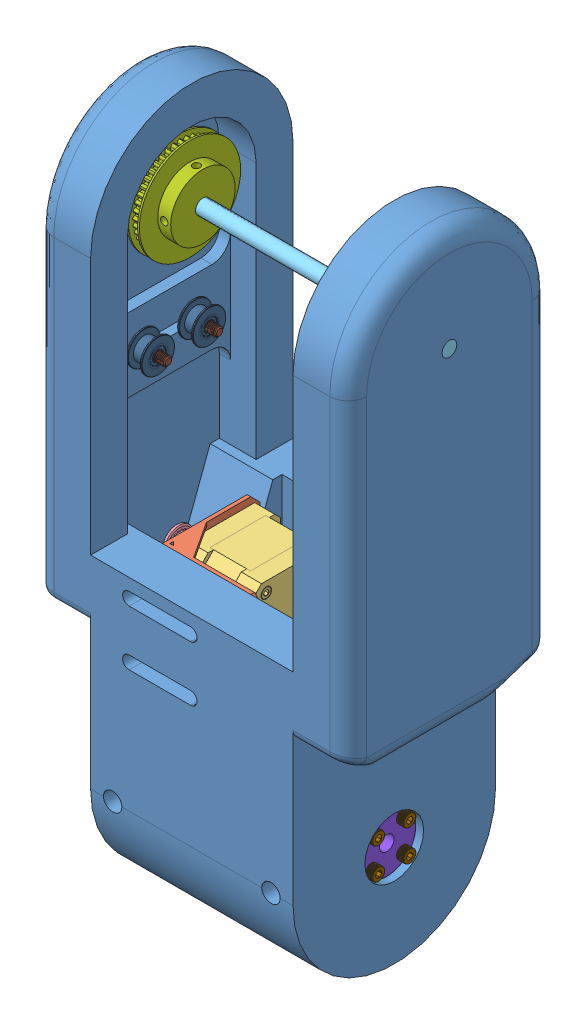
SolidWorks assembly Part2, configuration Default. Lengths in mm.
Overall size (170 359.61 110).
22 component instances, 11 part files, 45 mates.
Components (placement in the parent):
- Part2-1: Part2 [Default] at (184.7996 161.3802 267.2035) size (170 359.61 110)
- Nema17 motor support-1: Nema17 motor support [Default] at (88.827 136.3802 297.2035) x (1 0 0) z (0 1 0) size (53 51 50)
- nema17-34-1: nema17-34 [Default] at (154.696 127.2402 289.9023) x (0 0 -1) z (0 1 0) size (48.3 64 42.3)
- Puly GT2 20 trục 5mm-1: Puly GT2 20 trục 5mm [Конфигурация1] at (82.827 161.3802 267.2035) x (-1 0 0) z (0 0 1) size (16 16 16)
- bar_170mm-1: bar_170mm [Default] at (44.7996 325.9891 267.2035) x (0 0 -1) z (1 0 0) size (8 8 170)
- Ball Bearing 8mm I.D, 22mm O.D-1: Ball Bearing 8mm I.D, 22mm O.D [Default] at (51.2996 325.9891 267.2035) x (0 0 -1) z (1 0 0) size (22 22 7)
- Ball Bearing 8mm I.D, 22mm O.D-2: Ball Bearing 8mm I.D, 22mm O.D [Default] at (208.2996 325.9891 267.2035) x (0 -0.984808 0.173648) z (-1 0 0) size (22 22 7)
- Pulley 80 8mm-1: Pulley 80 8mm [Default] at (67.827 325.9891 267.2035) x (0 -1 0) z (0 0 1) size (55 14 55)
- Flange_8mm-1: Flange_8mm [Default] at (180.7996 76.3802 267.2035) x (0 0 1) z (0 -1 0) size (32 13 32)
- Flange_8mm-2: Flange_8mm [Default] at (78.7996 76.3802 267.2035) x (0 0 1) z (0 1 0) size (32 13 32)
- M4 CUP HEAD SCREW-1: M4 CUP HEAD SCREW [Default] at (88.7996 84.8655 258.7182) x (0 1 0) z (0 0 1) size (6.85 14.06 6.85)
- M4 CUP HEAD SCREW-4: M4 CUP HEAD SCREW [Default] at (88.7996 84.8655 275.6888) x (0 0.987351 0.158553) z (0 -0.158553 0.987351) size (6.85 14.06 6.85)
- M4 CUP HEAD SCREW-6: M4 CUP HEAD SCREW [Default] at (88.7996 67.895 275.6888) x (0 0.959125 0.282984) z (0 -0.282984 0.959125) size (6.85 14.06 6.85)
- M4 CUP HEAD SCREW-8: M4 CUP HEAD SCREW [Default] at (88.7996 67.895 258.7182) x (0 0.928571 0.371154) z (0 -0.371154 0.928571) size (6.85 14.06 6.85)
- M4 CUP HEAD SCREW-10: M4 CUP HEAD SCREW [Default] at (170.7996 84.8655 275.6888) x (0 0.642788 0.766044) z (0 0.766044 -0.642788) size (6.85 14.06 6.85)
- M4 CUP HEAD SCREW-12: M4 CUP HEAD SCREW [Default] at (170.7996 84.8655 258.7182) x (0 0.766044 0.642788) z (0 0.642788 -0.766044) size (6.85 14.06 6.85)
- M4 CUP HEAD SCREW-14: M4 CUP HEAD SCREW [Default] at (170.7996 67.895 258.7182) x (0 0.866025 0.5) z (0 0.5 -0.866025) size (6.85 14.06 6.85)
- M4 CUP HEAD SCREW-16: M4 CUP HEAD SCREW [Default] at (170.7996 67.895 275.6888) x (0 0.939693 0.34202) z (0 0.34202 -0.939693) size (6.85 14.06 6.85)
- GT2 - 20T_Tension Pulley Without Teeth+603ZZ _dzino-2: GT2 - 20T_Tension Pulley Without Teeth+603ZZ _dzino [Výchozí] at (69.2996 256.1847 279.9125) x (0 -0.248896 -0.96853) z (0 0.96853 -0.248896) size (18 8.5 18)
- GT2 - 20T_Tension Pulley Without Teeth+603ZZ _dzino-3: GT2 - 20T_Tension Pulley Without Teeth+603ZZ _dzino [Výchozí] at (69.2996 256.1847 252.0738) x (0 0.542384 -0.840131) z (0 0.840131 0.542384) size (18 8.5 18)
- M5x25-1: M5x25 [Default] at (44.7996 256.1847 252.0738) x (1 0 0) z (0 -0.923005 0.384788) size (30.03 8.5 8.5)
- M5x25-2: M5x25 [Default] at (44.7996 256.1847 279.9125) x (1 0 0) z (0 -0.972339 0.233576) size (30.03 8.5 8.5)
Mates (geometry in assembly coordinates):
- Coincident1: coincident anti-aligned: plane of Nema17 motor support-1 through (90.827 186.3802 246.2035) normal (1 0 0); plane of nema17-34-1 through (90.827 161.3802 267.2035) normal (-1 0 0)
- Concentric1: concentric aligned: cylinder of Nema17 motor support-1 through (88.827 161.3802 267.2035) axis (1 0 0) radius 11.05; cylinder of nema17-34-1 through (90.827 161.3802 267.2035) axis (1 0 0) radius 11
- Coincident2: coincident aligned: plane of nema17-34-1 through (66.827 161.3802 267.2035) normal (-1 0 0); plane of Puly GT2 20 trục 5mm-1 through (66.827 161.3802 267.2035) normal (-1 0 0)
- Concentric2: concentric anti-aligned: cylinder of nema17-34-1 through (90.827 161.3802 267.2035) axis (1 0 0) radius 2.5; cylinder of Puly GT2 20 trục 5mm-1 through (82.827 161.3802 267.2035) axis (-1 0 0) radius 2.5
- Coincident3: coincident anti-aligned: plane of Part2-1 through (88.827 136.3802 302.2035) normal (1 0 0); plane of Nema17 motor support-1 through (88.827 186.3802 297.2035) normal (-1 0 0)
- Coincident4: coincident anti-aligned: plane of Part2-1 through (184.7996 136.3802 267.2035) normal (0 1 0); plane of Nema17 motor support-1 through (88.827 136.3802 297.2035) normal (0 -1 0)
- Coincident5: coincident anti-aligned: plane of Part2-1 through (172.827 186.3802 297.2035) normal (0 0 -1); plane of Nema17 motor support-1 through (141.827 186.3802 297.2035) normal (0 0 1)
- Coincident6: coincident aligned: plane of Part2-1 through (47.7996 325.9891 267.2035) normal (1 0 0); circle of Ball Bearing 8mm I.D, 22mm O.D-1
- Concentric3: concentric anti-aligned: cylinder of Part2-1 through (47.7996 325.9891 267.2035) axis (1 0 0) radius 11; cylinder of Ball Bearing 8mm I.D, 22mm O.D-1 through (54.7996 325.9891 267.2035) axis (-1 0 0) radius 11
- Coincident7: coincident aligned: plane of Part2-1 through (211.7996 325.9891 267.2035) normal (-1 0 0); circle of Ball Bearing 8mm I.D, 22mm O.D-2
- Concentric4: concentric anti-aligned: cylinder of Part2-1 through (211.7996 325.9891 267.2035) axis (-1 0 0) radius 11; cylinder of Ball Bearing 8mm I.D, 22mm O.D-2 through (204.7996 325.9891 267.2035) axis (1 0 0) radius 11
- Concentric5: concentric aligned: cylinder of bar_170mm-1 through (214.7996 325.9891 267.2035) axis (-1 0 0) radius 4; cylinder of Ball Bearing 8mm I.D, 22mm O.D-1 through (54.7996 325.9891 267.2035) axis (-1 0 0) radius 4
- Coincident8: coincident aligned: plane of Part2-1 through (44.7996 325.9891 267.2035) normal (-1 0 0); plane of bar_170mm-1 through (44.7996 325.9891 267.2035) normal (-1 0 0)
- Concentric6: concentric anti-aligned: cylinder of bar_170mm-1 through (214.7996 325.9891 267.2035) axis (-1 0 0) radius 4; cylinder of Pulley 80 8mm-1 through (66.827 325.9891 267.2035) axis (1 0 0) radius 4
- Coincident9: coincident aligned: plane of Puly GT2 20 trục 5mm-1 through (66.827 161.3802 267.2035) normal (-1 0 0); plane of Pulley 80 8mm-1 through (66.827 325.9891 267.2035) normal (-1 0 0)
- Coincident10: coincident anti-aligned: plane of Part2-1 through (167.7996 76.3802 267.2035) normal (1 0 0); plane of Flange_8mm-1 through (167.7996 76.3802 267.2035) normal (-1 0 0)
- Concentric7: concentric aligned: cylinder of Part2-1 through (167.7996 76.3802 267.2035) axis (1 0 0) radius 8; cylinder of Flange_8mm-1 through (167.7996 76.3802 267.2035) axis (1 0 0) radius 8
- Coincident11: coincident anti-aligned: plane of Part2-1 through (91.7996 76.3802 267.2035) normal (-1 0 0); plane of Flange_8mm-2 through (91.7996 76.3802 267.2035) normal (1 0 0)
- Concentric8: concentric aligned: cylinder of Part2-1 through (81.7996 76.3802 267.2035) axis (-1 0 0) radius 16; cylinder of Flange_8mm-2 through (91.7996 76.3802 267.2035) axis (-1 0 0) radius 8
- Concentric9: concentric anti-aligned: cylinder of Part2-1 through (157.7996 84.8655 275.6888) axis (1 0 0) radius 2; cylinder of Flange_8mm-1 through (180.7996 84.8655 275.6888) axis (-1 0 0) radius 2
- Concentric10: concentric anti-aligned: cylinder of Part2-1 through (101.7996 84.8655 258.7182) axis (-1 0 0) radius 2; cylinder of Flange_8mm-2 through (78.7996 84.8655 258.7182) axis (1 0 0) radius 2
- Coincident12: coincident anti-aligned: plane of Flange_8mm-2 through (78.7996 76.3802 267.2035) normal (-1 0 0); plane of M4 CUP HEAD SCREW-1 through (78.7996 84.8655 258.7182) normal (1 0 0)
- Concentric11: concentric aligned: cylinder of Flange_8mm-2 through (78.7996 84.8655 258.7182) axis (1 0 0) radius 2; cylinder of M4 CUP HEAD SCREW-1 through (78.7996 84.8655 258.7182) axis (1 0 0) radius 2
- Coincident14: coincident anti-aligned: plane of Flange_8mm-2 through (78.7996 76.3802 267.2035) normal (-1 0 0); plane of M4 CUP HEAD SCREW-4 through (78.7996 84.8655 275.6888) normal (1 0 0)
- Concentric12: concentric aligned: cylinder of Flange_8mm-2 through (78.7996 84.8655 275.6888) axis (1 0 0) radius 2; cylinder of M4 CUP HEAD SCREW-4 through (78.7996 84.8655 275.6888) axis (1 0 0) radius 2
- Coincident15: coincident anti-aligned: plane of Flange_8mm-2 through (78.7996 76.3802 267.2035) normal (-1 0 0); plane of M4 CUP HEAD SCREW-6 through (78.7996 67.895 275.6888) normal (1 0 0)
- Concentric13: concentric aligned: cylinder of Flange_8mm-2 through (78.7996 67.895 275.6888) axis (1 0 0) radius 2; cylinder of M4 CUP HEAD SCREW-6 through (78.7996 67.895 275.6888) axis (1 0 0) radius 2
- Coincident16: coincident anti-aligned: plane of Flange_8mm-2 through (78.7996 76.3802 267.2035) normal (-1 0 0); plane of M4 CUP HEAD SCREW-8 through (78.7996 67.895 258.7182) normal (1 0 0)
- Concentric14: concentric aligned: cylinder of Flange_8mm-2 through (78.7996 67.895 258.7182) axis (1 0 0) radius 2; cylinder of M4 CUP HEAD SCREW-8 through (78.7996 67.895 258.7182) axis (1 0 0) radius 2
- Coincident17: coincident anti-aligned: plane of Flange_8mm-1 through (180.7996 76.3802 267.2035) normal (1 0 0); plane of M4 CUP HEAD SCREW-10 through (180.7996 84.8655 275.6888) normal (-1 0 0)
- Concentric15: concentric aligned: cylinder of Flange_8mm-1 through (180.7996 84.8655 275.6888) axis (-1 0 0) radius 2; cylinder of M4 CUP HEAD SCREW-10 through (180.7996 84.8655 275.6888) axis (-1 0 0) radius 2
- Coincident18: coincident anti-aligned: plane of Flange_8mm-1 through (180.7996 76.3802 267.2035) normal (1 0 0); plane of M4 CUP HEAD SCREW-12 through (180.7996 84.8655 258.7182) normal (-1 0 0)
- Concentric16: concentric aligned: cylinder of Flange_8mm-1 through (180.7996 84.8655 258.7182) axis (-1 0 0) radius 2; cylinder of M4 CUP HEAD SCREW-12 through (180.7996 84.8655 258.7182) axis (-1 0 0) radius 2
- Coincident19: coincident anti-aligned: plane of Flange_8mm-1 through (180.7996 76.3802 267.2035) normal (1 0 0); plane of M4 CUP HEAD SCREW-14 through (180.7996 67.895 258.7182) normal (-1 0 0)
- Concentric17: concentric aligned: cylinder of Flange_8mm-1 through (180.7996 67.895 258.7182) axis (-1 0 0) radius 2; cylinder of M4 CUP HEAD SCREW-14 through (180.7996 67.895 258.7182) axis (-1 0 0) radius 2
- Coincident20: coincident anti-aligned: plane of Flange_8mm-1 through (180.7996 76.3802 267.2035) normal (1 0 0); plane of M4 CUP HEAD SCREW-16 through (180.7996 67.895 275.6888) normal (-1 0 0)
- Concentric18: concentric aligned: cylinder of Flange_8mm-1 through (180.7996 67.895 275.6888) axis (-1 0 0) radius 2; cylinder of M4 CUP HEAD SCREW-16 through (180.7996 67.895 275.6888) axis (-1 0 0) radius 2
- Coincident22: coincident anti-aligned: plane of Part2-1 through (60.7996 161.3802 267.2035) normal (1 0 0); plane of GT2 - 20T_Tension Pulley Without Teeth+603ZZ _dzino-2 through (60.7996 256.1847 279.9125) normal (-1 0 0)
- Tangent5: tangent anti-aligned: plane of Part2-1 through (44.7996 253.6847 287.2035) normal (0 1 0); cylinder of GT2 - 20T_Tension Pulley Without Teeth+603ZZ _dzino-2 through (69.2996 256.1847 279.9125) axis (-1 0 0) radius 2.5
- Coincident23: coincident anti-aligned: plane of Part2-1 through (60.7996 161.3802 267.2035) normal (1 0 0); plane of GT2 - 20T_Tension Pulley Without Teeth+603ZZ _dzino-3 through (60.7996 256.1847 252.0738) normal (-1 0 0)
- Tangent6: tangent anti-aligned: plane of Part2-1 through (44.7996 253.6847 287.2035) normal (0 1 0); cylinder of GT2 - 20T_Tension Pulley Without Teeth+603ZZ _dzino-3 through (69.2996 256.1847 252.0738) axis (-1 0 0) radius 2.5
- Concentric20: concentric anti-aligned: cylinder of GT2 - 20T_Tension Pulley Without Teeth+603ZZ _dzino-3 through (60.7996 256.1847 252.0738) axis (1 0 0) radius 2.5; cylinder of M5x25-1 through (-43.9059 256.1847 252.0738) axis (-1 0 0) radius 2.488
- Coincident24: coincident anti-aligned: plane of Part2-1 through (49.7996 256.1847 287.2035) normal (-1 0 0); plane of M5x25-1 through (49.7996 257.142 254.3702) normal (1 0 0)
- Concentric21: concentric anti-aligned: cylinder of GT2 - 20T_Tension Pulley Without Teeth+603ZZ _dzino-2 through (60.7996 256.1847 279.9125) axis (1 0 0) radius 2.5; cylinder of M5x25-2 through (-43.9059 256.1847 279.9125) axis (-1 0 0) radius 2.488
- Coincident25: coincident anti-aligned: plane of Part2-1 through (49.7996 256.1847 287.2035) normal (-1 0 0); plane of M5x25-2 through (49.7996 256.7658 282.3317) normal (1 0 0)
